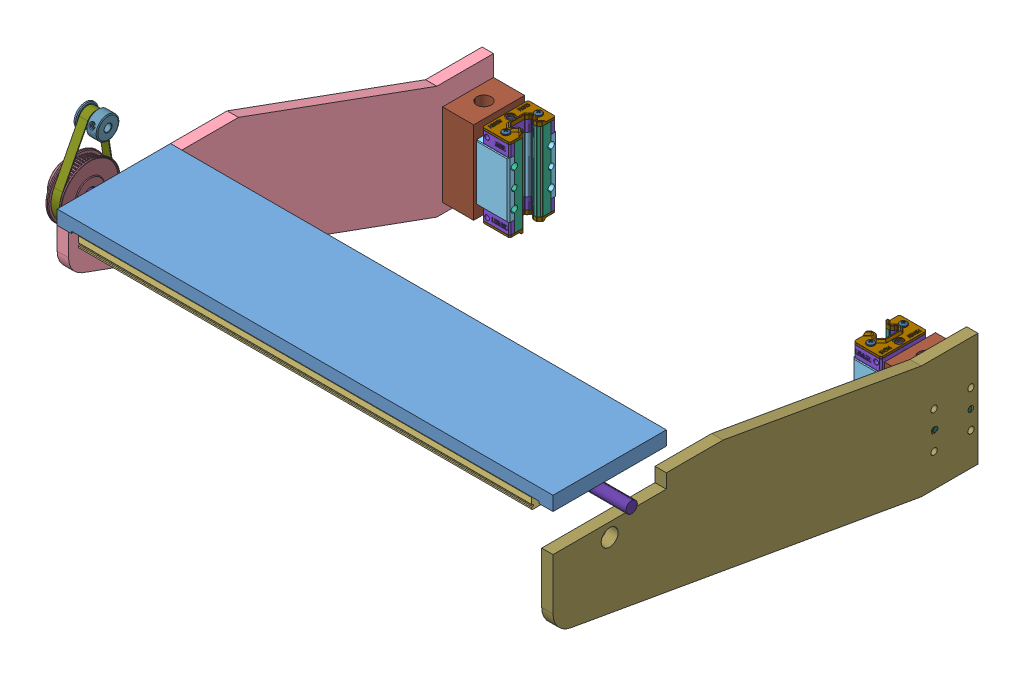
SolidWorks assembly Copia de Eje_X^Fresa_190502_2022, configuration Predeterminado. Lengths in mm.
Overall size (400 162.38 300).
40 component instances, 18 part files, 39 mates.
Components (placement in the parent):
- Puente_X^Copia de Eje_X_Fresa_190502_2022-1: Puente_X^Copia de Eje_X_Fresa_190502_2022 [Predeterminado] at (-189.2038 15.372 -72.2278) x (1 0 0) z (0 -1 0) size (350 80 10) (virtual)
- Copia de eje_X_guia_inf^Copia de Eje_X_Fresa_190502_2022-1: Copia de eje_X_guia_inf^Copia de Eje_X_Fresa_190502_2022 [Predeterminado] at (75.7962 2.9226 -66.2278) x (0 0 -1) z (-1 0 0) size (12 8.1 320) (virtual)
- Copia de eje_X_guia_sup^Copia de Eje_X_Fresa_190502_2022-1: Copia de eje_X_guia_sup^Copia de Eje_X_Fresa_190502_2022 [Predeterminado] at (-104.2038 2.9226 1.7722) x (0 0 1) z (1 0 0) size (12 8.1 320) (virtual)
-  Columa_xn^Copia de Eje_X_Fresa_190502_2022-1:  Columa_xn^Copia de Eje_X_Fresa_190502_2022 [Predeterminado] at (-181.2038 -35.5839 -292.2278) x (0 -1 0) z (-1 0 0) size (130.96 300 8) (virtual)
- Copia de HGH15CA^Copia de Eje_X_Fresa_190502_2022-1: Copia de HGH15CA^Copia de Eje_X_Fresa_190502_2022 [Default] at (-131.2038 -79.3839 -274.2278) x (0 0 -1) z (0 1 0) size (34 23.7 61.49) (virtual)
  - Copia de HGH15CA Block^Copia de HGH15CA_Copia de Eje_X_Fresa_190502_2022-1: Copia de HGH15CA Block^Copia de HGH15CA_Copia de Eje_X_Fresa_190502_2022 [HGR15R300CE20] at origin size (34 23.7 39.4) (virtual)
  - Copia de HGx15CA Retainer^Copia de HGH15CA_Copia de Eje_X_Fresa_190502_2022-1: Copia de HGx15CA Retainer^Copia de HGH15CA_Copia de Eje_X_Fresa_190502_2022 [HGR15R300CE20] at origin size (26 4 55.4) (virtual)
  - Copia de HGx15CA Tiny Red^Copia de HGH15CA_Copia de Eje_X_Fresa_190502_2022-1: Copia de HGx15CA Tiny Red^Copia de HGH15CA_Copia de Eje_X_Fresa_190502_2022 [HGR15R300CE20] at origin size (14.2 1 55.4) (virtual)
  - Copia de HGx15CA End Cap^Copia de HGH15CA_Copia de Eje_X_Fresa_190502_2022-1: Copia de HGx15CA End Cap^Copia de HGH15CA_Copia de Eje_X_Fresa_190502_2022 [HGR15R300CE20] at origin size (32.5 19.5 8) (virtual)
  - Copia de HGx15CA End Cap^Copia de HGH15CA_Copia de Eje_X_Fresa_190502_2022-2: Copia de HGx15CA End Cap^Copia de HGH15CA_Copia de Eje_X_Fresa_190502_2022 [HGR15R300CE20] x (-1 0 0) z (0 0 -1) size (32.5 19.5 8) (virtual)
  - Copia de HGx15CA Seal^Copia de HGH15CA_Copia de Eje_X_Fresa_190502_2022-1: Copia de HGx15CA Seal^Copia de HGH15CA_Copia de Eje_X_Fresa_190502_2022 [HGR15R300CE20] at origin size (32.5 19.5 3) (virtual)
  - Copia de HGx15CA Seal^Copia de HGH15CA_Copia de Eje_X_Fresa_190502_2022-2: Copia de HGx15CA Seal^Copia de HGH15CA_Copia de Eje_X_Fresa_190502_2022 [HGR15R300CE20] x (-1 0 0) z (0 0 -1) size (32.5 19.5 3) (virtual)
  - pan head cross recess screw_isog-1: pan head cross recess screw_isog [ISO 7045 - M2.5 x 16 - Z - 16C] at (11.5 11.8 30.8) x (0 0 -1) z (0 -1 0) size (18.05 5 5)
  - pan head cross recess screw_isog-2: pan head cross recess screw_isog [ISO 7045 - M2.5 x 16 - Z - 16C] at (-11.5 11.8 30.8) x (0 0 -1) z (0 1 0) size (18.05 5 5)
  - pan head cross recess screw_isog-3: pan head cross recess screw_isog [ISO 7045 - M2.5 x 16 - Z - 16C] at (11.5 11.8 -30.8) x (0 0 1) z (0 -1 0) size (18.05 5 5)
  - pan head cross recess screw_isog-4: pan head cross recess screw_isog [ISO 7045 - M2.5 x 16 - Z - 16C] at (-11.5 11.8 -30.8) x (0 0 1) z (0 1 0) size (18.05 5 5)
- Soporte_tuerca_husillo_X^Copia de Eje_X_Fresa_190502_2022-1: Soporte_tuerca_husillo_X^Copia de Eje_X_Fresa_190502_2022 [Predeterminado] at (-159.2038 -108.5839 -256.2278) x (0 1 0) z (-1 0 0) size (58.4 36 22) (virtual)
- Columa_xp^Copia de Eje_X_Fresa_190502_2022-1: Columa_xp^Copia de Eje_X_Fresa_190502_2022 [Predeterminado] at (160.7962 -35.5839 -292.2278) x (0 -1 0) z (-1 0 0) size (130.96 300 8) (virtual)
- Copia de HGH15CA^Copia de Eje_X_Fresa_190502_2022-2: Copia de HGH15CA^Copia de Eje_X_Fresa_190502_2022 [Default] at (102.7962 -79.3839 -274.2278) x (0 0 -1) z (0 -1 0) size (34 23.7 61.49) (virtual)
  - Copia de HGH15CA Block^Copia de HGH15CA_Copia de Eje_X_Fresa_190502_2022-1: Copia de HGH15CA Block^Copia de HGH15CA_Copia de Eje_X_Fresa_190502_2022 [HGR15R300CE20] at origin size (34 23.7 39.4) (virtual)
  - Copia de HGx15CA Retainer^Copia de HGH15CA_Copia de Eje_X_Fresa_190502_2022-1: Copia de HGx15CA Retainer^Copia de HGH15CA_Copia de Eje_X_Fresa_190502_2022 [HGR15R300CE20] at origin size (26 4 55.4) (virtual)
  - Copia de HGx15CA Tiny Red^Copia de HGH15CA_Copia de Eje_X_Fresa_190502_2022-1: Copia de HGx15CA Tiny Red^Copia de HGH15CA_Copia de Eje_X_Fresa_190502_2022 [HGR15R300CE20] at origin size (14.2 1 55.4) (virtual)
  - Copia de HGx15CA End Cap^Copia de HGH15CA_Copia de Eje_X_Fresa_190502_2022-1: Copia de HGx15CA End Cap^Copia de HGH15CA_Copia de Eje_X_Fresa_190502_2022 [HGR15R300CE20] at origin size (32.5 19.5 8) (virtual)
  - Copia de HGx15CA End Cap^Copia de HGH15CA_Copia de Eje_X_Fresa_190502_2022-2: Copia de HGx15CA End Cap^Copia de HGH15CA_Copia de Eje_X_Fresa_190502_2022 [HGR15R300CE20] x (-1 0 0) z (0 0 -1) size (32.5 19.5 8) (virtual)
  - Copia de HGx15CA Seal^Copia de HGH15CA_Copia de Eje_X_Fresa_190502_2022-1: Copia de HGx15CA Seal^Copia de HGH15CA_Copia de Eje_X_Fresa_190502_2022 [HGR15R300CE20] at origin size (32.5 19.5 3) (virtual)
  - Copia de HGx15CA Seal^Copia de HGH15CA_Copia de Eje_X_Fresa_190502_2022-2: Copia de HGx15CA Seal^Copia de HGH15CA_Copia de Eje_X_Fresa_190502_2022 [HGR15R300CE20] x (-1 0 0) z (0 0 -1) size (32.5 19.5 3) (virtual)
  - pan head cross recess screw_isog-1: pan head cross recess screw_isog [ISO 7045 - M2.5 x 16 - Z - 16C] at (11.5 11.8 30.8) x (0 0 -1) z (0 -1 0) size (18.05 5 5)
  - pan head cross recess screw_isog-2: pan head cross recess screw_isog [ISO 7045 - M2.5 x 16 - Z - 16C] at (-11.5 11.8 30.8) x (0 0 -1) z (0 1 0) size (18.05 5 5)
  - pan head cross recess screw_isog-3: pan head cross recess screw_isog [ISO 7045 - M2.5 x 16 - Z - 16C] at (11.5 11.8 -30.8) x (0 0 1) z (0 -1 0) size (18.05 5 5)
  - pan head cross recess screw_isog-4: pan head cross recess screw_isog [ISO 7045 - M2.5 x 16 - Z - 16C] at (-11.5 11.8 -30.8) x (0 0 1) z (0 1 0) size (18.05 5 5)
- Soporte_tuerca_husillo_X^Copia de Eje_X_Fresa_190502_2022-2: Soporte_tuerca_husillo_X^Copia de Eje_X_Fresa_190502_2022 [Predeterminado] at (130.7962 -50.1839 -256.2278) x (0 -1 0) z (1 0 0) size (58.4 36 22) (virtual)
- Copia de GT2_60T_8_6^Copia de Eje_X_Fresa_190502_2022-1: Copia de GT2_60T_8_6^Copia de Eje_X_Fresa_190502_2022 [Default] at (-216.1761 -4.128 -32.2278) x (0 0 1) z (1 0 0) size (42 42 18) (virtual)
- Copia de GT2_20T^Copia de Eje_X_Fresa_190502_2022-1: Copia de GT2_20T^Copia de Eje_X_Fresa_190502_2022 [Конфигурация1] at (-199.7261 36.3557 -38.7137) x (-1 0 0) z (0 0.380598 0.924741) size (16 16 16) (virtual)
- Copia de NEMA 23HS7430^Copia de Eje_X_Fresa_190502_2022-1: Copia de NEMA 23HS7430^Copia de Eje_X_Fresa_190502_2022 [По умолчанию] at (-187.6038 45.572 -50.4278) x (0 1 0) z (1 0 0) size (58.4 56.4 95.6) (hidden, virtual)
- guia_4x20^Copia de Eje_X_Fresa_190502_2022-1: guia_4x20^Copia de Eje_X_Fresa_190502_2022 [Predeterminado] at (-169.2038 -79.3839 -262.2278) x (0 0 1) z (-1 0 0) size (4 4 20) (virtual)
- guia_4x20^Copia de Eje_X_Fresa_190502_2022-2: guia_4x20^Copia de Eje_X_Fresa_190502_2022 [Predeterminado] at (-169.2038 -79.3839 -286.2278) x (0 0 1) z (-1 0 0) size (4 4 20) (virtual)
- Correa_158^Copia de Eje_X_Fresa_190502_2022-1: Correa_158^Copia de Eje_X_Fresa_190502_2022 [Predeterminado] at (-214.1761 -4.128 -32.2278) x (0 0.987408 -0.158192) z (1 0 0) size (66.95 38.7 6) (virtual)
- guia_4x20^Copia de Eje_X_Fresa_190502_2022-3: guia_4x20^Copia de Eje_X_Fresa_190502_2022 [Predeterminado] at (140.7962 -79.3839 -262.2278) x (0 -0.924225 -0.381849) z (1 0 0) size (4 4 20) (virtual)
- guia_4x20^Copia de Eje_X_Fresa_190502_2022-4: guia_4x20^Copia de Eje_X_Fresa_190502_2022 [Predeterminado] at (140.7962 -79.3839 -286.2278) x (0 -0.305624 0.952152) z (1 0 0) size (4 4 20) (virtual)
- Husillo^Copia de Eje_X_Fresa_190502_2022-1: Husillo^Copia de Eje_X_Fresa_190502_2022 [Predeterminado] at (176.3239 -4.128 -32.2278) x (0 0 1) z (-1 0 0) size (8 8 400) (virtual)
Mates (geometry in assembly coordinates):
- Coincidente8: coincident aligned: plane of Puente_X^Copia de Eje_X_Fresa_190502_2022-1 through (-189.2038 5.372 7.7722) normal (-1 0 0); plane of  Columa_xn^Copia de Eje_X_Fresa_190502_2022-1 through (-189.2038 -10.4485 -7.2278) normal (-1 0 0)
- Coincidente9: coincident anti-aligned: plane of Puente_X^Copia de Eje_X_Fresa_190502_2022-1 through (-189.2038 5.372 -72.2278) normal (0 -1 0); plane of  Columa_xn^Copia de Eje_X_Fresa_190502_2022-1 through (-189.2038 5.372 7.7722) normal (0 1 0)
- Coincidente10: coincident anti-aligned: plane of Puente_X^Copia de Eje_X_Fresa_190502_2022-1 through (160.7962 5.372 -72.2278) normal (0 0 -1); plane of  Columa_xn^Copia de Eje_X_Fresa_190502_2022-1 through (-189.2038 15.372 -72.2278) normal (0 0 1)
- Coincidente11: coincident aligned: plane of Puente_X^Copia de Eje_X_Fresa_190502_2022-1 through (160.7962 5.372 7.7722) normal (1 0 0); plane of Columa_xp^Copia de Eje_X_Fresa_190502_2022-1 through (160.7962 -10.4485 -7.2278) normal (1 0 0)
- Coincidente12: coincident anti-aligned: plane of Puente_X^Copia de Eje_X_Fresa_190502_2022-1 through (160.7962 5.372 -72.2278) normal (0 0 -1); plane of Columa_xp^Copia de Eje_X_Fresa_190502_2022-1 through (152.7962 15.372 -72.2278) normal (0 0 1)
- Coincidente13: coincident anti-aligned: plane of Puente_X^Copia de Eje_X_Fresa_190502_2022-1 through (-189.2038 5.372 -72.2278) normal (0 -1 0); plane of Columa_xp^Copia de Eje_X_Fresa_190502_2022-1 through (152.7962 5.372 7.7722) normal (0 1 0)
- Coincidente16: coincident aligned: plane of Puente_X^Copia de Eje_X_Fresa_190502_2022-1 through (160.7962 5.372 7.7722) normal (0 0 1); plane of Copia de eje_X_guia_sup^Copia de Eje_X_Fresa_190502_2022-1 through (145.7962 6.872 7.7722) normal (0 0 1)
- Coincidente32: coincident aligned: plane of Puente_X^Copia de Eje_X_Fresa_190502_2022-1 through (160.7962 5.372 -72.2278) normal (0 0 -1); plane of Copia de eje_X_guia_inf^Copia de Eje_X_Fresa_190502_2022-1 through (-174.2038 6.872 -72.2278) normal (0 0 -1)
- Coincidente33: coincident aligned: plane of Puente_X^Copia de Eje_X_Fresa_190502_2022-1 through (-189.2038 5.372 7.7722) normal (-1 0 0); plane of Copia de NEMA 23HS7430^Copia de Eje_X_Fresa_190502_2022-1 through (-189.2038 45.572 -50.4278) normal (-1 0 0)
- Distancia6: distance = 2 mm anti-aligned: plane of Copia de NEMA 23HS7430^Copia de Eje_X_Fresa_190502_2022-1 through (-177.6038 17.372 -78.6278) normal (0 -1 0); plane of Puente_X^Copia de Eje_X_Fresa_190502_2022-1 through (-189.2038 15.372 -72.2278) normal (0 1 0)
- Distancia7: distance = 30 mm aligned: plane of Copia de NEMA 23HS7430^Copia de Eje_X_Fresa_190502_2022-1 through (-177.6038 17.372 -22.2278) normal (0 0 1); plane of Puente_X^Copia de Eje_X_Fresa_190502_2022-1 through (160.7962 5.372 7.7722) normal (0 0 1)
- Coincidente42: coincident anti-aligned: plane of  Columa_xn^Copia de Eje_X_Fresa_190502_2022-1 through (-181.2038 -10.4485 -7.2278) normal (1 0 0); plane of Soporte_tuerca_husillo_X^Copia de Eje_X_Fresa_190502_2022-1 through (-181.2038 -108.5839 -256.2278) normal (-1 0 0)
- Distancia10: distance = 7 mm aligned: plane of Soporte_tuerca_husillo_X^Copia de Eje_X_Fresa_190502_2022-1 through (-181.2038 -108.5839 -256.2278) normal (0 -1 0); plane of  Columa_xn^Copia de Eje_X_Fresa_190502_2022-1 through (-189.2038 -115.5839 -292.2278) normal (0 -1 0)
- Coincidente44: coincident aligned: plane of  Columa_xn^Copia de Eje_X_Fresa_190502_2022-1 through (-189.2038 -35.5839 -292.2278) normal (0 0 -1); plane of Soporte_tuerca_husillo_X^Copia de Eje_X_Fresa_190502_2022-1 through (-181.2038 -108.5839 -292.2278) normal (0 0 -1)
- Coincidente45: coincident anti-aligned: plane of Copia de HGH15CA^Copia de Eje_X_Fresa_190502_2022-1/Copia de HGH15CA Block^Copia de HGH15CA_Copia de Eje_X_Fresa_190502_2022-1 through (-159.2038 -59.6839 -290.2278) normal (-1 0 0); plane of Soporte_tuerca_husillo_X^Copia de Eje_X_Fresa_190502_2022-1 through (-159.2038 -108.5839 -256.2278) normal (1 0 0)
- Distancia11: distance = 1 mm aligned: plane of Copia de HGH15CA^Copia de Eje_X_Fresa_190502_2022-1/Copia de HGH15CA Block^Copia de HGH15CA_Copia de Eje_X_Fresa_190502_2022-1 through (-136.5038 -59.6839 -291.2278) normal (0 0 -1); plane of Soporte_tuerca_husillo_X^Copia de Eje_X_Fresa_190502_2022-1 through (-181.2038 -108.5839 -292.2278) normal (0 0 -1)
- Coincidente47: coincident aligned: plane of Copia de HGH15CA^Copia de Eje_X_Fresa_190502_2022-1/Copia de HGx15CA Seal^Copia de HGH15CA_Copia de Eje_X_Fresa_190502_2022-2 through (-137.6195 -108.5839 -279.3778) normal (0 -1 0); plane of Soporte_tuerca_husillo_X^Copia de Eje_X_Fresa_190502_2022-1 through (-181.2038 -108.5839 -256.2278) normal (0 -1 0)
- Concéntrica7: concentric anti-aligned: cylinder of  Columa_xn^Copia de Eje_X_Fresa_190502_2022-1 through (-189.2038 -79.3839 -262.2278) axis (-1 0 0) radius 2; cylinder of guia_4x20^Copia de Eje_X_Fresa_190502_2022-1 through (-189.2038 -79.3839 -262.2278) axis (1 0 0) radius 2
- Coincidente48: coincident aligned: plane of  Columa_xn^Copia de Eje_X_Fresa_190502_2022-1 through (-189.2038 -10.4485 -7.2278) normal (-1 0 0); plane of guia_4x20^Copia de Eje_X_Fresa_190502_2022-1 through (-189.2038 -79.3839 -262.2278) normal (-1 0 0)
- Coincidente49: coincident aligned: plane of  Columa_xn^Copia de Eje_X_Fresa_190502_2022-1 through (-189.2038 -10.4485 -7.2278) normal (-1 0 0); plane of guia_4x20^Copia de Eje_X_Fresa_190502_2022-2 through (-189.2038 -79.3839 -286.2278) normal (-1 0 0)
- Concéntrica8: concentric anti-aligned: cylinder of  Columa_xn^Copia de Eje_X_Fresa_190502_2022-1 through (-189.2038 -79.3839 -286.2278) axis (-1 0 0) radius 2; cylinder of guia_4x20^Copia de Eje_X_Fresa_190502_2022-2 through (-189.2038 -79.3839 -286.2278) axis (1 0 0) radius 2
- Concéntrica9: concentric anti-aligned: cylinder of Correa_158^Copia de Eje_X_Fresa_190502_2022-1 through (-208.1761 -4.128 -32.2278) axis (-1 0 0) radius 18.85; cylinder of Copia de GT2_60T_8_6^Copia de Eje_X_Fresa_190502_2022-1 through (-223.6761 -4.128 -32.2278) axis (1 0 0) radius 12.5
- Distancia12: distance = 1 mm anti-aligned: plane of Correa_158^Copia de Eje_X_Fresa_190502_2022-1 through (-208.1761 -4.128 -32.2278) normal (1 0 0); plane of Copia de GT2_60T_8_6^Copia de Eje_X_Fresa_190502_2022-1 through (-207.1761 -4.128 -32.2278) normal (-1 0 0)
- Concéntrica10: concentric anti-aligned: cylinder of Copia de GT2_20T^Copia de Eje_X_Fresa_190502_2022-1 through (-199.7261 36.3557 -38.7137) axis (1 0 0) radius 8; cylinder of Correa_158^Copia de Eje_X_Fresa_190502_2022-1 through (-208.1761 36.3557 -38.7137) axis (-1 0 0) radius 6.1
- Distancia13: distance = 1 mm anti-aligned: plane of Correa_158^Copia de Eje_X_Fresa_190502_2022-1 through (-208.1761 -4.128 -32.2278) normal (1 0 0); plane of Copia de GT2_20T^Copia de Eje_X_Fresa_190502_2022-1 through (-207.1761 36.3557 -38.7137) normal (-1 0 0)
- Coincidente50: coincident anti-aligned: plane of Columa_xp^Copia de Eje_X_Fresa_190502_2022-1 through (152.7962 -10.4485 -7.2278) normal (-1 0 0); plane of Soporte_tuerca_husillo_X^Copia de Eje_X_Fresa_190502_2022-2 through (152.7962 -50.1839 -256.2278) normal (1 0 0)
- Coincidente51: coincident aligned: plane of Columa_xp^Copia de Eje_X_Fresa_190502_2022-1 through (152.7962 -35.5839 -292.2278) normal (0 0 -1); plane of Soporte_tuerca_husillo_X^Copia de Eje_X_Fresa_190502_2022-2 through (152.7962 -50.1839 -292.2278) normal (0 0 -1)
- Distancia14: distance = 7 mm aligned: plane of Soporte_tuerca_husillo_X^Copia de Eje_X_Fresa_190502_2022-2 through (152.7962 -108.5839 -256.2278) normal (0 -1 0); plane of Columa_xp^Copia de Eje_X_Fresa_190502_2022-1 through (152.7962 -115.5839 -292.2278) normal (0 -1 0)
- Distancia15: distance = 1 mm aligned: plane of Copia de HGH15CA^Copia de Eje_X_Fresa_190502_2022-2/Copia de HGH15CA Block^Copia de HGH15CA_Copia de Eje_X_Fresa_190502_2022-1 through (108.0962 -99.0839 -291.2278) normal (0 0 -1); plane of Soporte_tuerca_husillo_X^Copia de Eje_X_Fresa_190502_2022-2 through (152.7962 -50.1839 -292.2278) normal (0 0 -1)
- Coincidente55: coincident aligned: plane of Copia de HGH15CA^Copia de Eje_X_Fresa_190502_2022-2/Copia de HGx15CA Seal^Copia de HGH15CA_Copia de Eje_X_Fresa_190502_2022-1 through (109.2119 -108.5839 -269.0778) normal (0 -1 0); plane of Soporte_tuerca_husillo_X^Copia de Eje_X_Fresa_190502_2022-2 through (152.7962 -108.5839 -256.2278) normal (0 -1 0)
- Coincidente56: coincident aligned: plane of Columa_xp^Copia de Eje_X_Fresa_190502_2022-1 through (160.7962 -10.4485 -7.2278) normal (1 0 0); plane of guia_4x20^Copia de Eje_X_Fresa_190502_2022-3 through (160.7962 -79.3839 -262.2278) normal (1 0 0)
- Concéntrica11: concentric aligned: circle of Columa_xp^Copia de Eje_X_Fresa_190502_2022-1; circle of guia_4x20^Copia de Eje_X_Fresa_190502_2022-4
- Concéntrica12: concentric anti-aligned: cylinder of Columa_xp^Copia de Eje_X_Fresa_190502_2022-1 through (160.7962 -79.3839 -262.2278) axis (1 0 0) radius 2; cylinder of guia_4x20^Copia de Eje_X_Fresa_190502_2022-3 through (160.7962 -79.3839 -262.2278) axis (-1 0 0) radius 2
- Coincidente57: coincident aligned: plane of Columa_xp^Copia de Eje_X_Fresa_190502_2022-1 through (160.7962 -10.4485 -7.2278) normal (1 0 0); plane of guia_4x20^Copia de Eje_X_Fresa_190502_2022-4 through (160.7962 -79.3839 -286.2278) normal (1 0 0)
- Concéntrica13: concentric anti-aligned: cylinder of Copia de GT2_60T_8_6^Copia de Eje_X_Fresa_190502_2022-1 through (-186.1761 -4.128 -32.2278) axis (-1 0 0) radius 4; cylinder of Husillo^Copia de Eje_X_Fresa_190502_2022-1 through (-223.6761 -4.128 -32.2278) axis (1 0 0) radius 4
- Paralelo1: parallel aligned: plane of Copia de GT2_60T_8_6^Copia de Eje_X_Fresa_190502_2022-1 through (-219.9261 -4.128 -45.2278) normal (0 0 -1); plane of Husillo^Copia de Eje_X_Fresa_190502_2022-1 through (-213.6761 -8.128 -35.2278) normal (0 0 -1)
- Concéntrica14: concentric aligned: cylinder of  Columa_xn^Copia de Eje_X_Fresa_190502_2022-1 through (-189.2038 -4.128 -32.2278) axis (1 0 0) radius 6; cylinder of Husillo^Copia de Eje_X_Fresa_190502_2022-1 through (-223.6761 -4.128 -32.2278) axis (1 0 0) radius 4
- Coincidente59: coincident aligned: plane of Copia de GT2_60T_8_6^Copia de Eje_X_Fresa_190502_2022-1 through (-223.6761 -4.128 -32.2278) normal (-1 0 0); plane of Husillo^Copia de Eje_X_Fresa_190502_2022-1 through (-223.6761 -4.128 -32.2278) normal (-1 0 0)
- Paralelo2: parallel aligned: plane of  Columa_xn^Copia de Eje_X_Fresa_190502_2022-1 through (-189.2038 5.372 7.7722) normal (0 0 1); plane of Copia de GT2_60T_8_6^Copia de Eje_X_Fresa_190502_2022-1 through (-219.9261 -4.128 -19.2278) normal (0 0 1)
